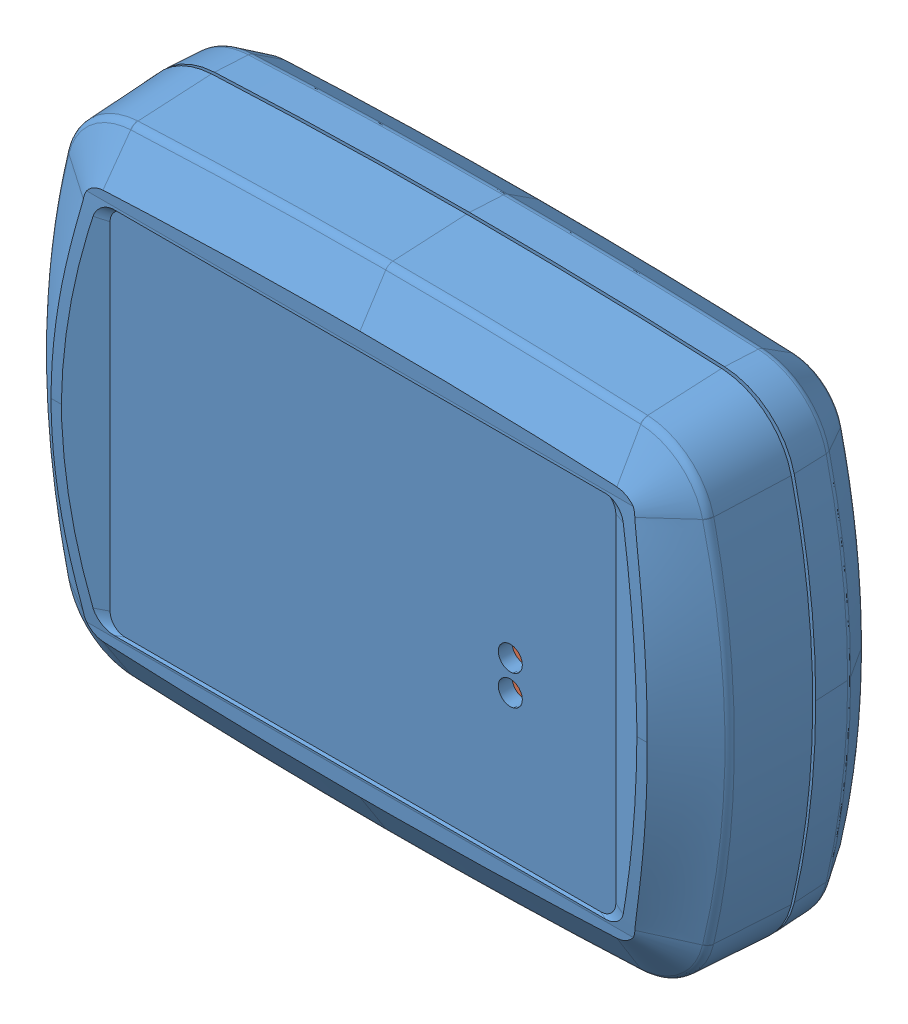
SolidWorks assembly СБ Peggy Receiver, configuration Default. Lengths in mm.
Overall size (116.83 83 32.04).
267 component instances, 109 part files, 3 mates.
Components (placement in the parent):
- G1910-1: G1910 [Default] at origin size (116.83 83 32.04)
- Печатная плата Peggy Receiver-1: Печатная плата Peggy Receiver [Default] at (11919.9713 53.7301 2.2215) x (0.000006 1 0) z (0 0 1) size (75.31 78.06 11.44)
  - Печатная плата Peggy Receiver(2)^Печатная плата Peggy Receiver-2: Печатная плата Peggy Receiver(2)^Печатная плата Peggy Receiver [Default] at origin size (75.31 78.06 11.44) (virtual)
    - Board^Печатная плата Peggy Receiver(2)_Печатная плата Peggy Receiver-2: Board^Печатная плата Peggy Receiver(2)_Печатная плата Peggy Receiver [Default] at origin size (73.81 76.5 0.41) (virtual)
      - Open CASCADE STEP translator 7.5 1.1.1^Board_Печатная плата Peggy Receiver(2)_Печатная плата Peggy Receiver-1: Open CASCADE STEP translator 7.5 1.1.1^Board_Печатная плата Peggy Receiver(2)_Печатная плата Peggy Receiver [Default] at (0 0 -0.4115) size (73.81 76.5 0.41) (virtual)
    - XW1^Печатная плата Peggy Receiver(2)_Печатная плата Peggy Receiver-2: XW1^Печатная плата Peggy Receiver(2)_Печатная плата Peggy Receiver [Default] at origin size (3.01 2.86 1.29) (virtual)
      - IPX^XW1_Печатная плата Peggy Receiver(2)_Печатная плата Peggy Receiver-1: IPX^XW1_Печатная плата Peggy Receiver(2)_Печатная плата Peggy Receiver [Default] at (14.0624 73.0251 1.27) x (0 1 0) z (0 0 1) size (3.01 2.86 1.29) (virtual)
    - D1^Печатная плата Peggy Receiver(2)_Печатная плата Peggy Receiver-2: D1^Печатная плата Peggy Receiver(2)_Печатная плата Peggy Receiver [Default] at origin size (15.7 37.6 11.44) (virtual)
      - HC-SERIES^D1_Печатная плата Peggy Receiver(2)_Печатная плата Peggy Receiver-1: HC-SERIES^D1_Печатная плата Peggy Receiver(2)_Печатная плата Peggy Receiver [Default] at (65.255 43.965 4) x (0 -1 0) z (-1 0 0) size (37.6 11.44 15.7) (virtual)
        - HC-SERIES.stp^HC-SERIES_D1_Печатная плата Peggy Receiver(2)_Печатная плата Peggy Receiver-1: HC-SERIES.stp^HC-SERIES_D1_Печатная плата Peggy Receiver(2)_Печатная плата Peggy Receiver [Default] at origin size (37.6 11.44 15.7) (virtual)
          - Assembly1.stp^HC-SERIES.stp_HC-SERIES_D1_Печатная плата Peggy Receiver(2)_Печатная плата Peggy Receiver-1: Assembly1.stp^HC-SERIES.stp_HC-SERIES_D1_Печатная плата Peggy Receiver(2)_Печатная плата Peggy Receiver [Default] at origin size (37.6 2.6 15.7) (virtual)
            - _______-________9.stp^Assembly1.stp_HC-SERIES.stp_HC-SERIES_D1_Печатная плата Peggy Receiver(2)_Печатная плата Peggy Receiver-1: _______-________9.stp^Assembly1.stp_HC-SERIES.stp_HC-SERIES_D1_Печатная плата Peggy Receiver(2)_Печатная плата Peggy Receiver [Default] at origin size (37.6 2.6 15.7) (virtual)
          - Assembly8.stp^HC-SERIES.stp_HC-SERIES_D1_Печатная плата Peggy Receiver(2)_Печатная плата Peggy Receiver-1: Assembly8.stp^HC-SERIES.stp_HC-SERIES_D1_Печатная плата Peggy Receiver(2)_Печатная плата Peggy Receiver [Default] at origin size (2.54 11.44 15.24) (virtual)
            - Pin Header 6 x 1 TH 2.54mm Pitch.stp^Assembly8.stp_HC-SERIES.stp_HC-SERIES_D1_Печатная плата Peggy Receiver(2)_Печатная плата Peggy Receiver-1: Pin Header 6 x 1 TH 2.54mm Pitch.stp^Assembly8.stp_HC-SERIES.stp_HC-SERIES_D1_Печатная плата Peggy Receiver(2)_Печатная плата Peggy Receiver [Default] at (1.3634 -4.0367 -6.3335) x (1 0 0) z (0 -1 0) size (0.64 0.64 11.43) (virtual)
            - Pin Header 6 x 1 TH 2.54mm Pitch-0.stp^Assembly8.stp_HC-SERIES.stp_HC-SERIES_D1_Печатная плата Peggy Receiver(2)_Печатная плата Peggy Receiver-1: Pin Header 6 x 1 TH 2.54mm Pitch-0.stp^Assembly8.stp_HC-SERIES.stp_HC-SERIES_D1_Печатная плата Peggy Receiver(2)_Печатная плата Peggy Receiver [Default] at (1.3634 -4.0367 -6.3335) x (1 0 0) z (0 -1 0) size (0.64 0.64 11.43) (virtual)
            - Pin Header 6 x 1 TH 2.54mm Pitch-1.stp^Assembly8.stp_HC-SERIES.stp_HC-SERIES_D1_Печатная плата Peggy Receiver(2)_Печатная плата Peggy Receiver-1: Pin Header 6 x 1 TH 2.54mm Pitch-1.stp^Assembly8.stp_HC-SERIES.stp_HC-SERIES_D1_Печатная плата Peggy Receiver(2)_Печатная плата Peggy Receiver [Default] at (1.3634 -4.0414 -6.3335) x (1 0 0) z (0 -1 0) size (0.64 0.64 11.43) (virtual)
            - Pin Header 6 x 1 TH 2.54mm Pitch-2.stp^Assembly8.stp_HC-SERIES.stp_HC-SERIES_D1_Печатная плата Peggy Receiver(2)_Печатная плата Peggy Receiver-1: Pin Header 6 x 1 TH 2.54mm Pitch-2.stp^Assembly8.stp_HC-SERIES.stp_HC-SERIES_D1_Печатная плата Peggy Receiver(2)_Печатная плата Peggy Receiver [Default] at (1.3634 -4.0354 -6.3335) x (1 0 0) z (0 -1 0) size (0.64 0.64 11.43) (virtual)
            - Pin Header 6 x 1 TH 2.54mm Pitch-3.stp^Assembly8.stp_HC-SERIES.stp_HC-SERIES_D1_Печатная плата Peggy Receiver(2)_Печатная плата Peggy Receiver-1: Pin Header 6 x 1 TH 2.54mm Pitch-3.stp^Assembly8.stp_HC-SERIES.stp_HC-SERIES_D1_Печатная плата Peggy Receiver(2)_Печатная плата Peggy Receiver [Default] at (1.3634 -4.0354 -6.3335) x (1 0 0) z (0 -1 0) size (0.64 0.63 11.43) (virtual)
            - Pin Header 6 x 1 TH 2.54mm Pitch-4.stp^Assembly8.stp_HC-SERIES.stp_HC-SERIES_D1_Печатная плата Peggy Receiver(2)_Печатная плата Peggy Receiver-1: Pin Header 6 x 1 TH 2.54mm Pitch-4.stp^Assembly8.stp_HC-SERIES.stp_HC-SERIES_D1_Печатная плата Peggy Receiver(2)_Печатная плата Peggy Receiver [Default] at (1.3634 -4.0354 -6.3335) x (1 0 0) z (0 -1 0) size (0.64 0.64 11.43) (virtual)
            - Pin Header 6 x 1 TH 2.54mm Pitch-5.stp^Assembly8.stp_HC-SERIES.stp_HC-SERIES_D1_Печатная плата Peggy Receiver(2)_Печатная плата Peggy Receiver-1: Pin Header 6 x 1 TH 2.54mm Pitch-5.stp^Assembly8.stp_HC-SERIES.stp_HC-SERIES_D1_Печатная плата Peggy Receiver(2)_Печатная плата Peggy Receiver [Default] at (1.3634 -1.5 -6.3335) x (1 0 0) z (0 -1 0) size (2.54 2.54 2.54) (virtual)
            - Pin Header 6 x 1 TH 2.54mm Pitch-6.stp^Assembly8.stp_HC-SERIES.stp_HC-SERIES_D1_Печатная плата Peggy Receiver(2)_Печатная плата Peggy Receiver-1: Pin Header 6 x 1 TH 2.54mm Pitch-6.stp^Assembly8.stp_HC-SERIES.stp_HC-SERIES_D1_Печатная плата Peggy Receiver(2)_Печатная плата Peggy Receiver [Default] at (1.3634 -1.5 -6.3335) x (1 0 0) z (0 -1 0) size (2.54 2.54 2.54) (virtual)
            - Pin Header 6 x 1 TH 2.54mm Pitch-7.stp^Assembly8.stp_HC-SERIES.stp_HC-SERIES_D1_Печатная плата Peggy Receiver(2)_Печатная плата Peggy Receiver-1: Pin Header 6 x 1 TH 2.54mm Pitch-7.stp^Assembly8.stp_HC-SERIES.stp_HC-SERIES_D1_Печатная плата Peggy Receiver(2)_Печатная плата Peggy Receiver [Default] at (1.3634 -1.5 -6.3335) x (1 0 0) z (0 -1 0) size (2.54 2.54 2.54) (virtual)
            - Pin Header 6 x 1 TH 2.54mm Pitch-8.stp^Assembly8.stp_HC-SERIES.stp_HC-SERIES_D1_Печатная плата Peggy Receiver(2)_Печатная плата Peggy Receiver-1: Pin Header 6 x 1 TH 2.54mm Pitch-8.stp^Assembly8.stp_HC-SERIES.stp_HC-SERIES_D1_Печатная плата Peggy Receiver(2)_Печатная плата Peggy Receiver [Default] at (1.3634 -1.5 -6.3335) x (1 0 0) z (0 -1 0) size (2.54 2.54 2.54) (virtual)
            - Pin Header 6 x 1 TH 2.54mm Pitch-9.stp^Assembly8.stp_HC-SERIES.stp_HC-SERIES_D1_Печатная плата Peggy Receiver(2)_Печатная плата Peggy Receiver-1: Pin Header 6 x 1 TH 2.54mm Pitch-9.stp^Assembly8.stp_HC-SERIES.stp_HC-SERIES_D1_Печатная плата Peggy Receiver(2)_Печатная плата Peggy Receiver [Default] at (1.3634 -1.5 -6.3335) x (1 0 0) z (0 -1 0) size (2.54 2.54 2.54) (virtual)
            - Pin Header 6 x 1 TH 2.54mm Pitch-10.stp^Assembly8.stp_HC-SERIES.stp_HC-SERIES_D1_Печатная плата Peggy Receiver(2)_Печатная плата Peggy Receiver-1: Pin Header 6 x 1 TH 2.54mm Pitch-10.stp^Assembly8.stp_HC-SERIES.stp_HC-SERIES_D1_Печатная плата Peggy Receiver(2)_Печатная плата Peggy Receiver [Default] at (1.3634 -1.5 -6.3335) x (1 0 0) z (0 -1 0) size (2.54 2.54 2.54) (virtual)
    - C13^Печатная плата Peggy Receiver(2)_Печатная плата Peggy Receiver-2: C13^Печатная плата Peggy Receiver(2)_Печатная плата Peggy Receiver [Default] at origin size (3.2 1.6 1) (virtual)
      - SW3dPS-1206 SMD Capacitor^C13_Печатная плата Peggy Receiver(2)_Печатная плата Peggy Receiver-1: SW3dPS-1206 SMD Capacitor^C13_Печатная плата Peggy Receiver(2)_Печатная плата Peggy Receiver [Default] at (19.609 14.0729 0) x (1 0 0) z (0 -1 0) size (3.2 1 1.6) (virtual)
    - C12^Печатная плата Peggy Receiver(2)_Печатная плата Peggy Receiver-2: C12^Печатная плата Peggy Receiver(2)_Печатная плата Peggy Receiver [Default] at origin size (3.2 1.6 1) (virtual)
      - SW3dPS-1206 SMD Capacitor^C12_Печатная плата Peggy Receiver(2)_Печатная плата Peggy Receiver-1: SW3dPS-1206 SMD Capacitor^C12_Печатная плата Peggy Receiver(2)_Печатная плата Peggy Receiver [Default] at (19.609 7.0729 0) x (1 0 0) z (0 -1 0) size (3.2 1 1.6) (virtual)
    - C11^Печатная плата Peggy Receiver(2)_Печатная плата Peggy Receiver-2: C11^Печатная плата Peggy Receiver(2)_Печатная плата Peggy Receiver [Default] at origin size (1.6 3.2 1) (virtual)
      - SW3dPS-1206 SMD Capacitor^C11_Печатная плата Peggy Receiver(2)_Печатная плата Peggy Receiver-1: SW3dPS-1206 SMD Capacitor^C11_Печатная плата Peggy Receiver(2)_Печатная плата Peggy Receiver [Default] at (12.6729 22.091 0) x (0 -1 0) z (-1 0 0) size (3.2 1 1.6) (virtual)
    - C6^Печатная плата Peggy Receiver(2)_Печатная плата Peggy Receiver-2: C6^Печатная плата Peggy Receiver(2)_Печатная плата Peggy Receiver [Default] at origin size (3.2 1.6 1) (virtual)
      - SW3dPS-1206 SMD Capacitor^C6_Печатная плата Peggy Receiver(2)_Печатная плата Peggy Receiver-1: SW3dPS-1206 SMD Capacitor^C6_Печатная плата Peggy Receiver(2)_Печатная плата Peggy Receiver [Default] at (60.4 45.7 0) x (1 0 0) z (0 -1 0) size (3.2 1 1.6) (virtual)
    - C5^Печатная плата Peggy Receiver(2)_Печатная плата Peggy Receiver-2: C5^Печатная плата Peggy Receiver(2)_Печатная плата Peggy Receiver [Default] at origin size (3.2 1.6 1) (virtual)
      - SW3dPS-1206 SMD Capacitor^C5_Печатная плата Peggy Receiver(2)_Печатная плата Peggy Receiver-1: SW3dPS-1206 SMD Capacitor^C5_Печатная плата Peggy Receiver(2)_Печатная плата Peggy Receiver [Default] at (32.309 24.6729 0) x (-1 0 0) z (0 1 0) size (3.2 1 1.6) (virtual)
    - C4^Печатная плата Peggy Receiver(2)_Печатная плата Peggy Receiver-2: C4^Печатная плата Peggy Receiver(2)_Печатная плата Peggy Receiver [Default] at origin size (1.6 3.2 1) (virtual)
      - SW3dPS-1206 SMD Capacitor^C4_Печатная плата Peggy Receiver(2)_Печатная плата Peggy Receiver-1: SW3dPS-1206 SMD Capacitor^C4_Печатная плата Peggy Receiver(2)_Печатная плата Peggy Receiver [Default] at (15 66.5 0) x (0 1 0) z (1 0 0) size (3.2 1 1.6) (virtual)
    - ZQ1^Печатная плата Peggy Receiver(2)_Печатная плата Peggy Receiver-2: ZQ1^Печатная плата Peggy Receiver(2)_Печатная плата Peggy Receiver [Default] at origin size (3.18 5 1.11) (virtual)
      - ABM3B^ZQ1_Печатная плата Peggy Receiver(2)_Печатная плата Peggy Receiver-1: ABM3B^ZQ1_Печатная плата Peggy Receiver(2)_Печатная плата Peggy Receiver [Default] at (27.6091 36.0728 0) x (0 1 0) z (1 0 0) size (5 1.11 3.17) (virtual)
    - X2^Печатная плата Peggy Receiver(2)_Печатная плата Peggy Receiver-2: X2^Печатная плата Peggy Receiver(2)_Печатная плата Peggy Receiver [Default] at origin size (5.43 8.2 3.3) (virtual)
      - User Library-MicroUSB-B_Molex_105017-0001^X2_Печатная плата Peggy Receiver(2)_Печатная плата Peggy Receiver-1: User Library-MicroUSB-B_Molex_105017-0001^X2_Печатная плата Peggy Receiver(2)_Печатная плата Peggy Receiver [Default] at (1.7 22.4 1.2) x (0 -1 0) z (-1 0 0) size (8.2 3.3 5.43) (virtual)
    - VD2^Печатная плата Peggy Receiver(2)_Печатная плата Peggy Receiver-2: VD2^Печатная плата Peggy Receiver(2)_Печатная плата Peggy Receiver [Default] at origin size (1.65 0.8 0.65) (virtual)
      - User Library-SOD523-2^VD2_Печатная плата Peggy Receiver(2)_Печатная плата Peggy Receiver-1: User Library-SOD523-2^VD2_Печатная плата Peggy Receiver(2)_Печатная плата Peggy Receiver [Default] at (26.8499 3.7999 0) x (0 1 0) z (1 0 0) size (0.8 0.65 1.65) (virtual)
    - VD1^Печатная плата Peggy Receiver(2)_Печатная плата Peggy Receiver-2: VD1^Печатная плата Peggy Receiver(2)_Печатная плата Peggy Receiver [Default] at origin size (0.81 1.61 0.61) (virtual)
      - User Library-LED_0603_R^VD1_Печатная плата Peggy Receiver(2)_Печатная плата Peggy Receiver-1: User Library-LED_0603_R^VD1_Печатная плата Peggy Receiver(2)_Печатная плата Peggy Receiver [Default] at (32.2999 13.773 0) x (0 1 0) z (0 0 1) size (1.61 0.81 0.61) (virtual)
        - User Library-LED_0603_R_Pocket002^User Library-LED_0603_R_VD1_Печатная плата Peggy Receiver(2)_Печатная плата Peggy Receiver-1: User Library-LED_0603_R_Pocket002^User Library-LED_0603_R_VD1_Печатная плата Peggy Receiver(2)_Печатная плата Peggy Receiver [Default] at origin size (0.41 0.81 0.21) (virtual)
        - User Library-LED_0603_R_Pad004^User Library-LED_0603_R_VD1_Печатная плата Peggy Receiver(2)_Печатная плата Peggy Receiver-1: User Library-LED_0603_R_Pad004^User Library-LED_0603_R_VD1_Печатная плата Peggy Receiver(2)_Печатная плата Peggy Receiver [Default] x (1 0 0) z (0 0 -1) size (0.4 0.8 0) (virtual)
        - User Library-LED_0603_R_Fillet^User Library-LED_0603_R_VD1_Печатная плата Peggy Receiver(2)_Печатная плата Peggy Receiver-1: User Library-LED_0603_R_Fillet^User Library-LED_0603_R_VD1_Печатная плата Peggy Receiver(2)_Печатная плата Peggy Receiver [Default] at origin size (1 0.7 0.4) (virtual)
        - User Library-LED_0603_R_Pocket001^User Library-LED_0603_R_VD1_Печатная плата Peggy Receiver(2)_Печатная плата Peggy Receiver-1: User Library-LED_0603_R_Pocket001^User Library-LED_0603_R_VD1_Печатная плата Peggy Receiver(2)_Печатная плата Peggy Receiver [Default] at origin size (0.4 0.8 0.2) (virtual)
        - User Library-LED_0603_R_Pad^User Library-LED_0603_R_VD1_Печатная плата Peggy Receiver(2)_Печатная плата Peggy Receiver-1: User Library-LED_0603_R_Pad^User Library-LED_0603_R_VD1_Печатная плата Peggy Receiver(2)_Печатная плата Peggy Receiver [Default] at origin size (0.8 0.8 0.2) (virtual)
    - U1^Печатная плата Peggy Receiver(2)_Печатная плата Peggy Receiver-2: U1^Печатная плата Peggy Receiver(2)_Печатная плата Peggy Receiver [Default] at origin size (3 2.8 1.4) (virtual)
      - AP2112K-3.3TRG1--3DModel-STEP-1^U1_Печатная плата Peggy Receiver(2)_Печатная плата Peggy Receiver-1: AP2112K-3.3TRG1--3DModel-STEP-1^U1_Печатная плата Peggy Receiver(2)_Печатная плата Peggy Receiver [Default] at (19.009 10.5729 0) x (-1 0 0) z (0 1 0) size (3 1.4 2.8) (virtual)
    - R9^Печатная плата Peggy Receiver(2)_Печатная плата Peggy Receiver-2: R9^Печатная плата Peggy Receiver(2)_Печатная плата Peggy Receiver [Default] at origin size (1.61 0.81 0.46) (virtual)
      - chip_0603_r^R9_Печатная плата Peggy Receiver(2)_Печатная плата Peggy Receiver-1: chip_0603_r^R9_Печатная плата Peggy Receiver(2)_Печатная плата Peggy Receiver [Default] at (9.4728 19.7911 0.21) x (0 1 0) z (0 0 1) size (0.81 1.61 0.46) (virtual)
    - R8^Печатная плата Peggy Receiver(2)_Печатная плата Peggy Receiver-2: R8^Печатная плата Peggy Receiver(2)_Печатная плата Peggy Receiver [Default] at origin size (0.81 1.61 0.46) (virtual)
      - chip_0603_r^R8_Печатная плата Peggy Receiver(2)_Печатная плата Peggy Receiver-1: chip_0603_r^R8_Печатная плата Peggy Receiver(2)_Печатная плата Peggy Receiver [Default] at (32.2999 11.0999 0.21) x (-1 0 0) z (0 0 1) size (0.81 1.61 0.46) (virtual)
    - R7^Печатная плата Peggy Receiver(2)_Печатная плата Peggy Receiver-2: R7^Печатная плата Peggy Receiver(2)_Печатная плата Peggy Receiver [Default] at origin size (0.81 1.61 0.46) (virtual)
      - chip_0603_r^R7_Печатная плата Peggy Receiver(2)_Печатная плата Peggy Receiver-1: chip_0603_r^R7_Печатная плата Peggy Receiver(2)_Печатная плата Peggy Receiver [Default] at (38.5089 45.7728 0.21) x (-1 0 0) z (0 0 1) size (0.81 1.61 0.46) (virtual)
    - R6^Печатная плата Peggy Receiver(2)_Печатная плата Peggy Receiver-2: R6^Печатная плата Peggy Receiver(2)_Печатная плата Peggy Receiver [Default] at origin size (0.9 1.7 0.55) (virtual)
      - 6665909488^R6_Печатная плата Peggy Receiver(2)_Печатная плата Peggy Receiver-1: 6665909488^R6_Печатная плата Peggy Receiver(2)_Печатная плата Peggy Receiver [Default] at (37.2999 10.5001 0) x (0 1 0) z (0 0 1) size (1.7 0.9 0.55) (virtual)
        - Terminal^6665909488_R6_Печатная плата Peggy Receiver(2)_Печатная плата Peggy Receiver-1: Terminal^6665909488_R6_Печатная плата Peggy Receiver(2)_Печатная плата Peggy Receiver [Default] at (-0.85 -0.45 0) size (0.1 0.9 0.55) (virtual)
          - Open CASCADE STEP translator 6.8 15.2.1^Terminal_6665909488_R6_Печатная плата Peggy Receiver(2)_Печатная плата Peggy Receiver-1: Open CASCADE STEP translator 6.8 15.2.1^Terminal_6665909488_R6_Печатная плата Peggy Receiver(2)_Печатная плата Peggy Receiver [Default] at origin size (0.1 0.9 0.55) (virtual)
        - Terminal^6665909488_R6_Печатная плата Peggy Receiver(2)_Печатная плата Peggy Receiver-2: Terminal^6665909488_R6_Печатная плата Peggy Receiver(2)_Печатная плата Peggy Receiver [Default] at (0.85 0.45 0) x (-1 0 0) z (0 0 1) size (0.1 0.9 0.55) (virtual)
          - Open CASCADE STEP translator 6.8 15.2.1^Terminal_6665909488_R6_Печатная плата Peggy Receiver(2)_Печатная плата Peggy Receiver-1: Open CASCADE STEP translator 6.8 15.2.1^Terminal_6665909488_R6_Печатная плата Peggy Receiver(2)_Печатная плата Peggy Receiver [Default] at origin size (0.1 0.9 0.55) (virtual)
        - Mid_Body^6665909488_R6_Печатная плата Peggy Receiver(2)_Печатная плата Peggy Receiver-1: Mid_Body^6665909488_R6_Печатная плата Peggy Receiver(2)_Печатная плата Peggy Receiver [Default] at (-0.85 -0.45 0) size (1.59 0.9 0.44) (virtual)
        - Mark^6665909488_R6_Печатная плата Peggy Receiver(2)_Печатная плата Peggy Receiver-1: Mark^6665909488_R6_Печатная плата Peggy Receiver(2)_Печатная плата Peggy Receiver [Default] at (-0.75 -0.45 0.495) size (1.5 0.9 0.06) (virtual)
    - R5^Печатная плата Peggy Receiver(2)_Печатная плата Peggy Receiver-2: R5^Печатная плата Peggy Receiver(2)_Печатная плата Peggy Receiver [Default] at origin size (0.81 1.61 0.46) (virtual)
      - chip_0603_r^R5_Печатная плата Peggy Receiver(2)_Печатная плата Peggy Receiver-1: chip_0603_r^R5_Печатная плата Peggy Receiver(2)_Печатная плата Peggy Receiver [Default] at (40.3089 45.7728 0.21) x (-1 0 0) z (0 0 1) size (0.81 1.61 0.46) (virtual)
    - R4^Печатная плата Peggy Receiver(2)_Печатная плата Peggy Receiver-2: R4^Печатная плата Peggy Receiver(2)_Печатная плата Peggy Receiver [Default] at origin size (0.81 1.61 0.46) (virtual)
      - chip_0603_r^R4_Печатная плата Peggy Receiver(2)_Печатная плата Peggy Receiver-1: chip_0603_r^R4_Печатная плата Peggy Receiver(2)_Печатная плата Peggy Receiver [Default] at (47.0089 38.8728 0.21) x (-1 0 0) z (0 0 1) size (0.81 1.61 0.46) (virtual)
    - R3^Печатная плата Peggy Receiver(2)_Печатная плата Peggy Receiver-2: R3^Печатная плата Peggy Receiver(2)_Печатная плата Peggy Receiver [Default] at origin size (0.9 1.7 0.55) (virtual)
      - 6665909808^R3_Печатная плата Peggy Receiver(2)_Печатная плата Peggy Receiver-1: 6665909808^R3_Печатная плата Peggy Receiver(2)_Печатная плата Peggy Receiver [Default] at (35.3001 66.2999 0) x (0 -1 0) z (0 0 1) size (1.7 0.9 0.55) (virtual)
        - Terminal-1^6665909808_R3_Печатная плата Peggy Receiver(2)_Печатная плата Peggy Receiver-1: Terminal-1^6665909808_R3_Печатная плата Peggy Receiver(2)_Печатная плата Peggy Receiver [Default] at (-0.85 -0.45 0) size (0.1 0.9 0.55) (virtual)
          - Open CASCADE STEP translator 6.8 15.2.1-0^Terminal-1_6665909808_R3_Печатная плата Peggy Receiver(2)_Печатная плата Peggy Receiver-1: Open CASCADE STEP translator 6.8 15.2.1-0^Terminal-1_6665909808_R3_Печатная плата Peggy Receiver(2)_Печатная плата Peggy Receiver [Default] at origin size (0.1 0.9 0.55) (virtual)
        - Terminal-1^6665909808_R3_Печатная плата Peggy Receiver(2)_Печатная плата Peggy Receiver-2: Terminal-1^6665909808_R3_Печатная плата Peggy Receiver(2)_Печатная плата Peggy Receiver [Default] at (0.85 0.45 0) x (-1 0 0) z (0 0 1) size (0.1 0.9 0.55) (virtual)
          - Open CASCADE STEP translator 6.8 15.2.1-0^Terminal-1_6665909808_R3_Печатная плата Peggy Receiver(2)_Печатная плата Peggy Receiver-1: Open CASCADE STEP translator 6.8 15.2.1-0^Terminal-1_6665909808_R3_Печатная плата Peggy Receiver(2)_Печатная плата Peggy Receiver [Default] at origin size (0.1 0.9 0.55) (virtual)
        - Mid_Body-1^6665909808_R3_Печатная плата Peggy Receiver(2)_Печатная плата Peggy Receiver-1: Mid_Body-1^6665909808_R3_Печатная плата Peggy Receiver(2)_Печатная плата Peggy Receiver [Default] at (-0.85 -0.45 0) size (1.59 0.9 0.44) (virtual)
        - Mark-2^6665909808_R3_Печатная плата Peggy Receiver(2)_Печатная плата Peggy Receiver-1: Mark-2^6665909808_R3_Печатная плата Peggy Receiver(2)_Печатная плата Peggy Receiver [Default] at (-0.75 -0.45 0.495) size (1.5 0.9 0.06) (virtual)
    - R2^Печатная плата Peggy Receiver(2)_Печатная плата Peggy Receiver-2: R2^Печатная плата Peggy Receiver(2)_Печатная плата Peggy Receiver [Default] at origin size (1.61 0.81 0.46) (virtual)
      - chip_0603_r^R2_Печатная плата Peggy Receiver(2)_Печатная плата Peggy Receiver-1: chip_0603_r^R2_Печатная плата Peggy Receiver(2)_Печатная плата Peggy Receiver [Default] at (48.7091 37.3728 0.21) x (0 -1 0) z (0 0 1) size (0.81 1.61 0.46) (virtual)
    - R1^Печатная плата Peggy Receiver(2)_Печатная плата Peggy Receiver-2: R1^Печатная плата Peggy Receiver(2)_Печатная плата Peggy Receiver [Default] at origin size (1.61 0.81 0.46) (virtual)
      - chip_0603_r^R1_Печатная плата Peggy Receiver(2)_Печатная плата Peggy Receiver-1: chip_0603_r^R1_Печатная плата Peggy Receiver(2)_Печатная плата Peggy Receiver [Default] at (30.4089 43.473 0.21) x (0 1 0) z (0 0 1) size (0.81 1.61 0.46) (virtual)
    - MPU1^Печатная плата Peggy Receiver(2)_Печатная плата Peggy Receiver-2: MPU1^Печатная плата Peggy Receiver(2)_Печатная плата Peggy Receiver [Default] at origin size (14.96 12 1.2) (virtual)
      - 6665910048^MPU1_Печатная плата Peggy Receiver(2)_Печатная плата Peggy Receiver-1: 6665910048^MPU1_Печатная плата Peggy Receiver(2)_Печатная плата Peggy Receiver [Default] at (37.5091 35.7228 0) x (0 -1 0) z (0 0 1) size (12 14.96 1.2) (virtual)
        - Body^6665910048_MPU1_Печатная плата Peggy Receiver(2)_Печатная плата Peggy Receiver-1: Body^6665910048_MPU1_Печатная плата Peggy Receiver(2)_Печатная плата Peggy Receiver [Default] at (-5 -5 0) size (10.01 10.01 1.15) (virtual)
          - Open CASCADE STEP translator 6.8 62.2.1^Body_6665910048_MPU1_Печатная плата Peggy Receiver(2)_Печатная плата Peggy Receiver-1: Open CASCADE STEP translator 6.8 62.2.1^Body_6665910048_MPU1_Печатная плата Peggy Receiver(2)_Печатная плата Peggy Receiver [Default] at origin size (10.01 10.01 1.15) (virtual)
        - Open CASCADE STEP translator 6.8 62.1^6665910048_MPU1_Печатная плата Peggy Receiver(2)_Печатная плата Peggy Receiver-1: Open CASCADE STEP translator 6.8 62.1^6665910048_MPU1_Печатная плата Peggy Receiver(2)_Печатная плата Peggy Receiver [Default] at (-5 -5 0.001) size (1.26 1.26 0.01) (virtual)
        - Leader^6665910048_MPU1_Печатная плата Peggy Receiver(2)_Печатная плата Peggy Receiver-1: Leader^6665910048_MPU1_Печатная плата Peggy Receiver(2)_Печатная плата Peggy Receiver [Default] at (-5 -4 0) x (-1 0 0) z (0 0 1) size (1 0.38 0.68) (virtual)
        - Leader^6665910048_MPU1_Печатная плата Peggy Receiver(2)_Печатная плата Peggy Receiver-2: Leader^6665910048_MPU1_Печатная плата Peggy Receiver(2)_Печатная плата Peggy Receiver [Default] at (-5 -3.2 0) x (-1 0 0) z (0 0 1) size (1 0.38 0.68) (virtual)
        - Leader^6665910048_MPU1_Печатная плата Peggy Receiver(2)_Печатная плата Peggy Receiver-3: Leader^6665910048_MPU1_Печатная плата Peggy Receiver(2)_Печатная плата Peggy Receiver [Default] at (-5 -2.4 0) x (-1 0 0) z (0 0 1) size (1 0.38 0.68) (virtual)
        - Leader^6665910048_MPU1_Печатная плата Peggy Receiver(2)_Печатная плата Peggy Receiver-4: Leader^6665910048_MPU1_Печатная плата Peggy Receiver(2)_Печатная плата Peggy Receiver [Default] at (-5 -1.6 0) x (-1 0 0) z (0 0 1) size (1 0.38 0.68) (virtual)
        - Leader^6665910048_MPU1_Печатная плата Peggy Receiver(2)_Печатная плата Peggy Receiver-5: Leader^6665910048_MPU1_Печатная плата Peggy Receiver(2)_Печатная плата Peggy Receiver [Default] at (-5 -0.8 0) x (-1 0 0) z (0 0 1) size (1 0.38 0.68) (virtual)
        - Leader^6665910048_MPU1_Печатная плата Peggy Receiver(2)_Печатная плата Peggy Receiver-6: Leader^6665910048_MPU1_Печатная плата Peggy Receiver(2)_Печатная плата Peggy Receiver [Default] at (-5 0 0) x (-1 0 0) z (0 0 1) size (1 0.38 0.68) (virtual)
        - Leader^6665910048_MPU1_Печатная плата Peggy Receiver(2)_Печатная плата Peggy Receiver-7: Leader^6665910048_MPU1_Печатная плата Peggy Receiver(2)_Печатная плата Peggy Receiver [Default] at (-5 0.8 0) x (-1 0 0) z (0 0 1) size (1 0.38 0.68) (virtual)
        - Leader^6665910048_MPU1_Печатная плата Peggy Receiver(2)_Печатная плата Peggy Receiver-8: Leader^6665910048_MPU1_Печатная плата Peggy Receiver(2)_Печатная плата Peggy Receiver [Default] at (-5 1.6 0) x (-1 0 0) z (0 0 1) size (1 0.38 0.68) (virtual)
        - Leader^6665910048_MPU1_Печатная плата Peggy Receiver(2)_Печатная плата Peggy Receiver-9: Leader^6665910048_MPU1_Печатная плата Peggy Receiver(2)_Печатная плата Peggy Receiver [Default] at (-5 2.4 0) x (-1 0 0) z (0 0 1) size (1 0.38 0.68) (virtual)
        - Leader^6665910048_MPU1_Печатная плата Peggy Receiver(2)_Печатная плата Peggy Receiver-10: Leader^6665910048_MPU1_Печатная плата Peggy Receiver(2)_Печатная плата Peggy Receiver [Default] at (-5 3.2 0) x (-1 0 0) z (0 0 1) size (1 0.38 0.68) (virtual)
        - Leader^6665910048_MPU1_Печатная плата Peggy Receiver(2)_Печатная плата Peggy Receiver-11: Leader^6665910048_MPU1_Печатная плата Peggy Receiver(2)_Печатная плата Peggy Receiver [Default] at (-5 4 0) x (-1 0 0) z (0 0 1) size (1 0.38 0.68) (virtual)
        - Leader^6665910048_MPU1_Печатная плата Peggy Receiver(2)_Печатная плата Peggy Receiver-12: Leader^6665910048_MPU1_Печатная плата Peggy Receiver(2)_Печатная плата Peggy Receiver [Default] at (5 -4 0) size (1 0.38 0.68) (virtual)
        - Leader^6665910048_MPU1_Печатная плата Peggy Receiver(2)_Печатная плата Peggy Receiver-13: Leader^6665910048_MPU1_Печатная плата Peggy Receiver(2)_Печатная плата Peggy Receiver [Default] at (5 -3.2 0) size (1 0.38 0.68) (virtual)
        - Leader^6665910048_MPU1_Печатная плата Peggy Receiver(2)_Печатная плата Peggy Receiver-14: Leader^6665910048_MPU1_Печатная плата Peggy Receiver(2)_Печатная плата Peggy Receiver [Default] at (5 -2.4 0) size (1 0.38 0.68) (virtual)
        - Leader^6665910048_MPU1_Печатная плата Peggy Receiver(2)_Печатная плата Peggy Receiver-15: Leader^6665910048_MPU1_Печатная плата Peggy Receiver(2)_Печатная плата Peggy Receiver [Default] at (5 -1.6 0) size (1 0.38 0.68) (virtual)
        - Leader^6665910048_MPU1_Печатная плата Peggy Receiver(2)_Печатная плата Peggy Receiver-16: Leader^6665910048_MPU1_Печатная плата Peggy Receiver(2)_Печатная плата Peggy Receiver [Default] at (5 -0.8 0) size (1 0.38 0.68) (virtual)
        - Leader^6665910048_MPU1_Печатная плата Peggy Receiver(2)_Печатная плата Peggy Receiver-17: Leader^6665910048_MPU1_Печатная плата Peggy Receiver(2)_Печатная плата Peggy Receiver [Default] at (5 0 0) size (1 0.38 0.68) (virtual)
        - Leader^6665910048_MPU1_Печатная плата Peggy Receiver(2)_Печатная плата Peggy Receiver-18: Leader^6665910048_MPU1_Печатная плата Peggy Receiver(2)_Печатная плата Peggy Receiver [Default] at (5 0.8 0) size (1 0.38 0.68) (virtual)
        - Leader^6665910048_MPU1_Печатная плата Peggy Receiver(2)_Печатная плата Peggy Receiver-19: Leader^6665910048_MPU1_Печатная плата Peggy Receiver(2)_Печатная плата Peggy Receiver [Default] at (5 1.6 0) size (1 0.38 0.68) (virtual)
        - Leader^6665910048_MPU1_Печатная плата Peggy Receiver(2)_Печатная плата Peggy Receiver-20: Leader^6665910048_MPU1_Печатная плата Peggy Receiver(2)_Печатная плата Peggy Receiver [Default] at (5 2.4 0) size (1 0.38 0.68) (virtual)
        - Leader^6665910048_MPU1_Печатная плата Peggy Receiver(2)_Печатная плата Peggy Receiver-21: Leader^6665910048_MPU1_Печатная плата Peggy Receiver(2)_Печатная плата Peggy Receiver [Default] at (5 3.2 0) size (1 0.38 0.68) (virtual)
        - Leader^6665910048_MPU1_Печатная плата Peggy Receiver(2)_Печатная плата Peggy Receiver-22: Leader^6665910048_MPU1_Печатная плата Peggy Receiver(2)_Печатная плата Peggy Receiver [Default] at (5 4 0) size (1 0.38 0.68) (virtual)
        - Leader-3^6665910048_MPU1_Печатная плата Peggy Receiver(2)_Печатная плата Peggy Receiver-1: Leader-3^6665910048_MPU1_Печатная плата Peggy Receiver(2)_Печатная плата Peggy Receiver [Default] at (-4 -5 0) x (0 -1 0) z (0 0 1) size (1 0.38 0.68) (virtual)
        - Leader-3^6665910048_MPU1_Печатная плата Peggy Receiver(2)_Печатная плата Peggy Receiver-2: Leader-3^6665910048_MPU1_Печатная плата Peggy Receiver(2)_Печатная плата Peggy Receiver [Default] at (-3.2 -5 0) x (0 -1 0) z (0 0 1) size (1 0.38 0.68) (virtual)
        - Leader-3^6665910048_MPU1_Печатная плата Peggy Receiver(2)_Печатная плата Peggy Receiver-3: Leader-3^6665910048_MPU1_Печатная плата Peggy Receiver(2)_Печатная плата Peggy Receiver [Default] at (-2.4 -5 0) x (0 -1 0) z (0 0 1) size (1 0.38 0.68) (virtual)
        - Leader-3^6665910048_MPU1_Печатная плата Peggy Receiver(2)_Печатная плата Peggy Receiver-4: Leader-3^6665910048_MPU1_Печатная плата Peggy Receiver(2)_Печатная плата Peggy Receiver [Default] at (-1.6 -5 0) x (0 -1 0) z (0 0 1) size (1 0.38 0.68) (virtual)
        - Leader-3^6665910048_MPU1_Печатная плата Peggy Receiver(2)_Печатная плата Peggy Receiver-5: Leader-3^6665910048_MPU1_Печатная плата Peggy Receiver(2)_Печатная плата Peggy Receiver [Default] at (-0.8 -5 0) x (0 -1 0) z (0 0 1) size (1 0.38 0.68) (virtual)
        - Leader-3^6665910048_MPU1_Печатная плата Peggy Receiver(2)_Печатная плата Peggy Receiver-6: Leader-3^6665910048_MPU1_Печатная плата Peggy Receiver(2)_Печатная плата Peggy Receiver [Default] at (0 -5 0) x (0 -1 0) z (0 0 1) size (1 0.38 0.68) (virtual)
        - Leader-3^6665910048_MPU1_Печатная плата Peggy Receiver(2)_Печатная плата Peggy Receiver-7: Leader-3^6665910048_MPU1_Печатная плата Peggy Receiver(2)_Печатная плата Peggy Receiver [Default] at (0.8 -5 0) x (0 -1 0) z (0 0 1) size (1 0.38 0.68) (virtual)
        - Leader-3^6665910048_MPU1_Печатная плата Peggy Receiver(2)_Печатная плата Peggy Receiver-8: Leader-3^6665910048_MPU1_Печатная плата Peggy Receiver(2)_Печатная плата Peggy Receiver [Default] at (1.6 -5 0) x (0 -1 0) z (0 0 1) size (1 0.38 0.68) (virtual)
        - Leader-3^6665910048_MPU1_Печатная плата Peggy Receiver(2)_Печатная плата Peggy Receiver-9: Leader-3^6665910048_MPU1_Печатная плата Peggy Receiver(2)_Печатная плата Peggy Receiver [Default] at (2.4 -5 0) x (0 -1 0) z (0 0 1) size (1 0.38 0.68) (virtual)
        - Leader-3^6665910048_MPU1_Печатная плата Peggy Receiver(2)_Печатная плата Peggy Receiver-10: Leader-3^6665910048_MPU1_Печатная плата Peggy Receiver(2)_Печатная плата Peggy Receiver [Default] at (3.2 -5 0) x (0 -1 0) z (0 0 1) size (1 0.38 0.68) (virtual)
        - Leader-3^6665910048_MPU1_Печатная плата Peggy Receiver(2)_Печатная плата Peggy Receiver-11: Leader-3^6665910048_MPU1_Печатная плата Peggy Receiver(2)_Печатная плата Peggy Receiver [Default] at (4 -5 0) x (0 -1 0) z (0 0 1) size (1 0.38 0.68) (virtual)
        - Leader-3^6665910048_MPU1_Печатная плата Peggy Receiver(2)_Печатная плата Peggy Receiver-12: Leader-3^6665910048_MPU1_Печатная плата Peggy Receiver(2)_Печатная плата Peggy Receiver [Default] at (-4 5 0) x (0 1 0) z (0 0 1) size (1 0.38 0.68) (virtual)
        - Leader-3^6665910048_MPU1_Печатная плата Peggy Receiver(2)_Печатная плата Peggy Receiver-13: Leader-3^6665910048_MPU1_Печатная плата Peggy Receiver(2)_Печатная плата Peggy Receiver [Default] at (-3.2 5 0) x (0 1 0) z (0 0 1) size (1 0.38 0.68) (virtual)
        - Leader-3^6665910048_MPU1_Печатная плата Peggy Receiver(2)_Печатная плата Peggy Receiver-14: Leader-3^6665910048_MPU1_Печатная плата Peggy Receiver(2)_Печатная плата Peggy Receiver [Default] at (-2.4 5 0) x (0 1 0) z (0 0 1) size (1 0.38 0.68) (virtual)
        - Leader-3^6665910048_MPU1_Печатная плата Peggy Receiver(2)_Печатная плата Peggy Receiver-15: Leader-3^6665910048_MPU1_Печатная плата Peggy Receiver(2)_Печатная плата Peggy Receiver [Default] at (-1.6 5 0) x (0 1 0) z (0 0 1) size (1 0.38 0.68) (virtual)
        - Leader-3^6665910048_MPU1_Печатная плата Peggy Receiver(2)_Печатная плата Peggy Receiver-16: Leader-3^6665910048_MPU1_Печатная плата Peggy Receiver(2)_Печатная плата Peggy Receiver [Default] at (-0.8 5 0) x (0 1 0) z (0 0 1) size (1 0.38 0.68) (virtual)
        - Leader-3^6665910048_MPU1_Печатная плата Peggy Receiver(2)_Печатная плата Peggy Receiver-17: Leader-3^6665910048_MPU1_Печатная плата Peggy Receiver(2)_Печатная плата Peggy Receiver [Default] at (0 5 0) x (0 1 0) z (0 0 1) size (1 0.38 0.68) (virtual)
        - Leader-3^6665910048_MPU1_Печатная плата Peggy Receiver(2)_Печатная плата Peggy Receiver-18: Leader-3^6665910048_MPU1_Печатная плата Peggy Receiver(2)_Печатная плата Peggy Receiver [Default] at (0.8 5 0) x (0 1 0) z (0 0 1) size (1 0.38 0.68) (virtual)
        - Leader-3^6665910048_MPU1_Печатная плата Peggy Receiver(2)_Печатная плата Peggy Receiver-19: Leader-3^6665910048_MPU1_Печатная плата Peggy Receiver(2)_Печатная плата Peggy Receiver [Default] at (1.6 5 0) x (0 1 0) z (0 0 1) size (1 0.38 0.68) (virtual)
        - Leader-3^6665910048_MPU1_Печатная плата Peggy Receiver(2)_Печатная плата Peggy Receiver-20: Leader-3^6665910048_MPU1_Печатная плата Peggy Receiver(2)_Печатная плата Peggy Receiver [Default] at (2.4 5 0) x (0 1 0) z (0 0 1) size (1 0.38 0.68) (virtual)
        - Leader-3^6665910048_MPU1_Печатная плата Peggy Receiver(2)_Печатная плата Peggy Receiver-21: Leader-3^6665910048_MPU1_Печатная плата Peggy Receiver(2)_Печатная плата Peggy Receiver [Default] at (3.2 5 0) x (0 1 0) z (0 0 1) size (1 0.38 0.68) (virtual)
        - Leader-3^6665910048_MPU1_Печатная плата Peggy Receiver(2)_Печатная плата Peggy Receiver-22: Leader-3^6665910048_MPU1_Печатная плата Peggy Receiver(2)_Печатная плата Peggy Receiver [Default] at (4 5 0) x (0 1 0) z (0 0 1) size (1 0.38 0.68) (virtual)
      - User Library-VQFN(44)^MPU1_Печатная плата Peggy Receiver(2)_Печатная плата Peggy Receiver-1: User Library-VQFN(44)^MPU1_Печатная плата Peggy Receiver(2)_Печатная плата Peggy Receiver [Default] at (33.963 32.1998 0) x (1 0 0) z (0 -1 0) size (7.1 0.95 7.1) (virtual)
    - L3^Печатная плата Peggy Receiver(2)_Печатная плата Peggy Receiver-2: L3^Печатная плата Peggy Receiver(2)_Печатная плата Peggy Receiver [Default] at origin size (1.25 2 0.85) (virtual)
      - User Library-FB_2012-1^L3_Печатная плата Peggy Receiver(2)_Печатная плата Peggy Receiver-1: User Library-FB_2012-1^L3_Печатная плата Peggy Receiver(2)_Печатная плата Peggy Receiver [Default] at (55.7999 44.8001 0) x (0 1 0) z (0 0 1) size (2 1.25 0.85) (virtual)
        - User Library-FB_2012-1_Pad001^User Library-FB_2012-1_L3_Печатная плата Peggy Receiver(2)_Печатная плата Peggy Receiver-1: User Library-FB_2012-1_Pad001^User Library-FB_2012-1_L3_Печатная плата Peggy Receiver(2)_Печатная плата Peggy Receiver [Default] at (0 0 0.03) size (1.94 1.19 0.79) (virtual)
        - User Library-FB_2012-1_Cut^User Library-FB_2012-1_L3_Печатная плата Peggy Receiver(2)_Печатная плата Peggy Receiver-1: User Library-FB_2012-1_Cut^User Library-FB_2012-1_L3_Печатная плата Peggy Receiver(2)_Печатная плата Peggy Receiver [Default] at origin size (2 1.25 0.85) (virtual)
    - L2^Печатная плата Peggy Receiver(2)_Печатная плата Peggy Receiver-2: L2^Печатная плата Peggy Receiver(2)_Печатная плата Peggy Receiver [Default] at origin size (2 1.25 0.85) (virtual)
      - User Library-FB_2012-1^L2_Печатная плата Peggy Receiver(2)_Печатная плата Peggy Receiver-1: User Library-FB_2012-1^L2_Печатная плата Peggy Receiver(2)_Печатная плата Peggy Receiver [Default] at (32.8001 22.2001 0) x (1 0 0) z (0 0 1) size (2 1.25 0.85) (virtual)
        - User Library-FB_2012-1_Pad001^User Library-FB_2012-1_L2_Печатная плата Peggy Receiver(2)_Печатная плата Peggy Receiver-1: User Library-FB_2012-1_Pad001^User Library-FB_2012-1_L2_Печатная плата Peggy Receiver(2)_Печатная плата Peggy Receiver [Default] at (0 0 0.03) size (1.94 1.19 0.79) (virtual)
        - User Library-FB_2012-1_Cut^User Library-FB_2012-1_L2_Печатная плата Peggy Receiver(2)_Печатная плата Peggy Receiver-1: User Library-FB_2012-1_Cut^User Library-FB_2012-1_L2_Печатная плата Peggy Receiver(2)_Печатная плата Peggy Receiver [Default] at origin size (2 1.25 0.85) (virtual)
    - L1^Печатная плата Peggy Receiver(2)_Печатная плата Peggy Receiver-2: L1^Печатная плата Peggy Receiver(2)_Печатная плата Peggy Receiver [Default] at origin size (2 1.25 0.85) (virtual)
      - User Library-FB_2012-1^L1_Печатная плата Peggy Receiver(2)_Печатная плата Peggy Receiver-1: User Library-FB_2012-1^L1_Печатная плата Peggy Receiver(2)_Печатная плата Peggy Receiver [Default] at (11.5999 64.8999 0) x (-1 0 0) z (0 0 1) size (2 1.25 0.85) (virtual)
        - User Library-FB_2012-1_Pad001^User Library-FB_2012-1_L1_Печатная плата Peggy Receiver(2)_Печатная плата Peggy Receiver-1: User Library-FB_2012-1_Pad001^User Library-FB_2012-1_L1_Печатная плата Peggy Receiver(2)_Печатная плата Peggy Receiver [Default] at (0 0 0.03) size (1.94 1.19 0.79) (virtual)
        - User Library-FB_2012-1_Cut^User Library-FB_2012-1_L1_Печатная плата Peggy Receiver(2)_Печатная плата Peggy Receiver-1: User Library-FB_2012-1_Cut^User Library-FB_2012-1_L1_Печатная плата Peggy Receiver(2)_Печатная плата Peggy Receiver [Default] at origin size (2 1.25 0.85) (virtual)
    - HL1^Печатная плата Peggy Receiver(2)_Печатная плата Peggy Receiver-2: HL1^Печатная плата Peggy Receiver(2)_Печатная плата Peggy Receiver [Default] at origin size (0.81 1.61 0.61) (virtual)
      - User Library-LED_0603_G^HL1_Печатная плата Peggy Receiver(2)_Печатная плата Peggy Receiver-1: User Library-LED_0603_G^HL1_Печатная плата Peggy Receiver(2)_Печатная плата Peggy Receiver [Default] at (37.2999 13.773 0) x (0 1 0) z (0 0 1) size (1.61 0.81 0.61) (virtual)
        - User Library-LED_0603_G_Pocket002^User Library-LED_0603_G_HL1_Печатная плата Peggy Receiver(2)_Печатная плата Peggy Receiver-1: User Library-LED_0603_G_Pocket002^User Library-LED_0603_G_HL1_Печатная плата Peggy Receiver(2)_Печатная плата Peggy Receiver [Default] at origin size (0.41 0.81 0.21) (virtual)
        - User Library-LED_0603_G_Pad004^User Library-LED_0603_G_HL1_Печатная плата Peggy Receiver(2)_Печатная плата Peggy Receiver-1: User Library-LED_0603_G_Pad004^User Library-LED_0603_G_HL1_Печатная плата Peggy Receiver(2)_Печатная плата Peggy Receiver [Default] x (1 0 0) z (0 0 -1) size (0.4 0.8 0) (virtual)
        - User Library-LED_0603_G_Fillet^User Library-LED_0603_G_HL1_Печатная плата Peggy Receiver(2)_Печатная плата Peggy Receiver-1: User Library-LED_0603_G_Fillet^User Library-LED_0603_G_HL1_Печатная плата Peggy Receiver(2)_Печатная плата Peggy Receiver [Default] at origin size (1 0.7 0.4) (virtual)
        - User Library-LED_0603_G_Pocket001^User Library-LED_0603_G_HL1_Печатная плата Peggy Receiver(2)_Печатная плата Peggy Receiver-1: User Library-LED_0603_G_Pocket001^User Library-LED_0603_G_HL1_Печатная плата Peggy Receiver(2)_Печатная плата Peggy Receiver [Default] at origin size (0.4 0.8 0.2) (virtual)
        - User Library-LED_0603_G_Pad^User Library-LED_0603_G_HL1_Печатная плата Peggy Receiver(2)_Печатная плата Peggy Receiver-1: User Library-LED_0603_G_Pad^User Library-LED_0603_G_HL1_Печатная плата Peggy Receiver(2)_Печатная плата Peggy Receiver [Default] at origin size (0.8 0.8 0.2) (virtual)
    - DD1^Печатная плата Peggy Receiver(2)_Печатная плата Peggy Receiver-2: DD1^Печатная плата Peggy Receiver(2)_Печатная плата Peggy Receiver [Default] at origin size (16 15.9 2.23) (virtual)
      - User Library-RFM96W^DD1_Печатная плата Peggy Receiver(2)_Печатная плата Peggy Receiver-1: User Library-RFM96W^DD1_Печатная плата Peggy Receiver(2)_Печатная плата Peggy Receiver [Default] at (17.298 57.975 1.15) x (1 0 0) z (0 0 1) size (16 15.9 2.23) (virtual)
        - Designator4^User Library-RFM96W_DD1_Печатная плата Peggy Receiver(2)_Печатная плата Peggy Receiver-1: Designator4^User Library-RFM96W_DD1_Печатная плата Peggy Receiver(2)_Печатная плата Peggy Receiver [Default] at origin size (0.5 1 0.5) (virtual)
          - Cap0402^Designator4_User Library-RFM96W_DD1_Печатная плата Peggy Receiver(2)_Печатная плата Peggy Receiver-1: Cap0402^Designator4_User Library-RFM96W_DD1_Печатная плата Peggy Receiver(2)_Печатная плата Peggy Receiver [Default] at (13.208 1.27 0) x (0 -1 0) z (-1 0 0) size (1 0.5 0.5) (virtual)
        - Designator6^User Library-RFM96W_DD1_Печатная плата Peggy Receiver(2)_Печатная плата Peggy Receiver-1: Designator6^User Library-RFM96W_DD1_Печатная плата Peggy Receiver(2)_Печатная плата Peggy Receiver [Default] at origin size (1 0.5 0.5) (virtual)
          - Cap0402^Designator6_User Library-RFM96W_DD1_Печатная плата Peggy Receiver(2)_Печатная плата Peggy Receiver-1: Cap0402^Designator6_User Library-RFM96W_DD1_Печатная плата Peggy Receiver(2)_Печатная плата Peggy Receiver [Default] at (7.239 1.143 0) x (-1 0 0) z (0 1 0) size (1 0.5 0.5) (virtual)
        - Designator7^User Library-RFM96W_DD1_Печатная плата Peggy Receiver(2)_Печатная плата Peggy Receiver-1: Designator7^User Library-RFM96W_DD1_Печатная плата Peggy Receiver(2)_Печатная плата Peggy Receiver [Default] at origin size (0.5 1 0.5) (virtual)
          - Cap0402^Designator7_User Library-RFM96W_DD1_Печатная плата Peggy Receiver(2)_Печатная плата Peggy Receiver-1: Cap0402^Designator7_User Library-RFM96W_DD1_Печатная плата Peggy Receiver(2)_Печатная плата Peggy Receiver [Default] at (3.81 5.08 0) x (0 -1 0) z (-1 0 0) size (1 0.5 0.5) (virtual)
        - Designator8^User Library-RFM96W_DD1_Печатная плата Peggy Receiver(2)_Печатная плата Peggy Receiver-1: Designator8^User Library-RFM96W_DD1_Печатная плата Peggy Receiver(2)_Печатная плата Peggy Receiver [Default] at origin size (1 0.5 0.5) (virtual)
          - Cap0402^Designator8_User Library-RFM96W_DD1_Печатная плата Peggy Receiver(2)_Печатная плата Peggy Receiver-1: Cap0402^Designator8_User Library-RFM96W_DD1_Печатная плата Peggy Receiver(2)_Печатная плата Peggy Receiver [Default] at (5.4 5.45 0) x (1 0 0) z (0 -1 0) size (1 0.5 0.5) (virtual)
